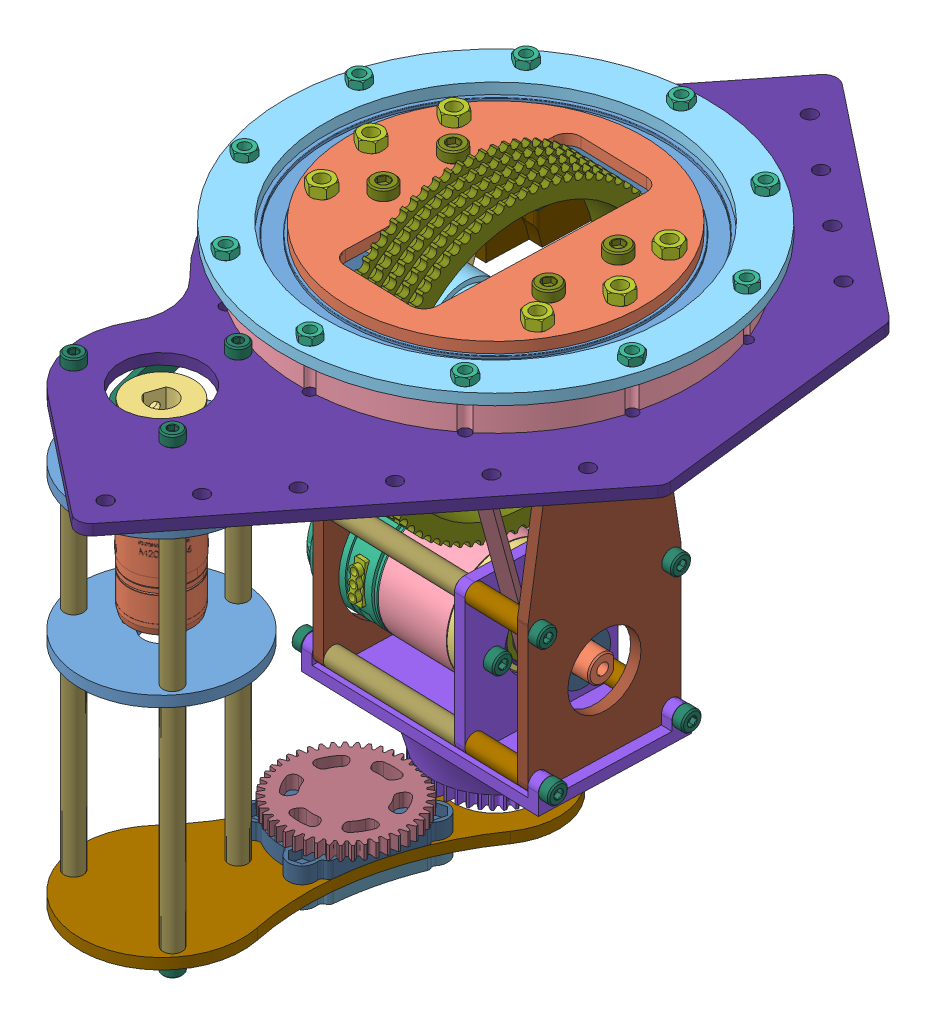
SolidWorks assembly 舵轮装配, configuration 默认. Lengths in mm.
Overall size (293.56 219.24 297.58).
150 component instances, 58 part files, 247 mates.
Components (placement in the parent):
- am-0198 4in Plaction Wheel-1: am-0198 4in Plaction Wheel [默认] at (-23.1352 -37.2288 84.5309) x (-0.999547 0 -0.03008) z (-0.012763 0.90552 0.424112)
  - am-0198 4in Plaction Wheel(2)^am-0198 4in Plaction Wheel-1: am-0198 4in Plaction Wheel(2)^am-0198 4in Plaction Wheel [默认] at origin (virtual)
- HRB 61821薄圈轴承-1: HRB 61821薄圈轴承 [默认] at (-8.689 -8.0564 92.8497) size (130 13 130)
- 舵轮底板-1: 舵轮底板 [默认] at (-8.689 4.9436 92.8497) x (-0.03008 0 0.999547) z (-0.999547 0 -0.03008) size (109 4 109)
- 舵轮侧面支撑-1: 舵轮侧面支撑 [默认] at (-38.1757 4.9436 91.9624) x (0.999547 0 0.03008) z (0.03008 0 -0.999547) size (14 45 35)
- 65齿 3m同步轮_舵轮定制板-1: 65齿 3m同步轮_舵轮定制板 [默认] at (11.9556 -30.0564 93.471) x (-0.028085 -0.358129 0.933249) z (0.999547 0 0.03008) size (62.3 62.3 8)
- 轮子轴承安装件-1: 轮子轴承安装件 [默认] at (-20.0339 -30.0564 92.5083) x (0.018247 -0.794989 -0.606349) z (0.023913 0.606624 -0.794629) size (28.1 11.65 28.1)
- 22 8 7轴承-1: 22 8 7轴承 [默认] at (-23.1825 -30.0564 92.4136) x (0.999547 0 0.03008) z (-0.028413 -0.328241 0.944167) size (7 25 25)
- 22 8 7轴承-2: 22 8 7轴承 [默认] at (12.9552 -30.0564 93.5011) x (-0.999547 0 -0.03008) z (0.029756 -0.146481 -0.988766) size (7 25 25)
- 舵轮用钢轴-1: 舵轮用钢轴 [默认] at (-43.1734 -30.0564 91.812) x (0.011091 0.929546 -0.368539) z (0.027961 -0.368706 -0.929125) size (8 70 8)
- 舵轮侧面支撑B-1: 舵轮侧面支撑B [默认] at (24.7958 4.9436 93.8574) x (-0.999547 0 -0.03008) z (-0.03008 0 0.999547) size (8 45 35)
- 舵轮轴承契合垫-1: 舵轮轴承契合垫 [默认] at (-8.689 -8.0564 92.8497) x (0.999547 0 0.03008) z (-0.03008 0 0.999547) size (18.69 13 65.65)
- 舵轮上底板-1: 舵轮上底板 [默认] at (-8.689 -12.0564 92.8497) x (-0.03008 0 0.999547) z (-0.999547 0 -0.03008) size (120 4 120)
- M3508电机安装板-1: M3508电机安装板 [默认] at (28.794 -7.5564 93.9777) x (0 1 0) z (0.03008 0 -0.999547) size (145.98 4 55)
- RoboMaster M3508直流无刷减速电-1: RoboMaster M3508直流无刷减速电 [默认] at (-82.126 -108.2793 108.2339) x (-0.011386 -0.925598 0.378336) z (0.999547 0 0.03008) size (77.46 77.46 98.4)
  - RoboMaster M3508直流无刷减速电 (1).STEP-1: RoboMaster M3508直流无刷减速电 (1).STEP [默认] at origin size (77.46 77.46 98.4)
    - 4_ASM_1.STEP-1: 4_ASM_1.STEP [默认] at (-1.7887 18.2683 39.841) x (-0.923508 0.383579 0) z (0.383579 0.923508 0) size (13.16 4.26 21.29)
      - __-__10_1__1.STEP-1: __-__10_1__1.STEP [默认] at origin size (2.4 2.3 2.24)
      - __-__10_3__1.STEP-1: __-__10_3__1.STEP [默认] at origin size (2.4 2.3 2.24)
      - __-__10_2__1.STEP-1: __-__10_2__1.STEP [默认] at origin size (2.4 2.3 2.24)
      - __-__20_1.STEP-1: __-__20_1.STEP [默认] at origin size (5.92 4.26 12.18)
    - 2_ASM.STEP-1: 2_ASM.STEP [默认] at (-1.7887 18.2683 50.441) x (-0.378508 0.925598 0) z (0.925598 0.378508 0) size (59.4 67.29 59.4)
      - 26_ASM.STEP-1: 26_ASM.STEP [默认] at (0 34.5 0) x (-0.381788 0 0.92425) z (-0.92425 0 -0.381788) size (22 6 22)
        - 28_1.STEP-1: 28_1.STEP [默认] at (0 2.5 0) size (20 0.2 20)
        - 27_1.STEP-1: 27_1.STEP [默认] at origin size (22 6 22)
        - 28_1.STEP-2: 28_1.STEP [默认] at (0 -2.7 0) size (20 0.2 20)
      - 26_ASM-1.STEP-1: 26_ASM-1.STEP [默认] at (0 27 0) x (-0.381788 0 0.92425) z (-0.92425 0 -0.381788) size (22 6 22)
        - 28_1.STEP-1: 28_1.STEP [默认] at (0 2.5 0) size (20 0.2 20)
        - 27_1.STEP-1: 27_1.STEP [默认] at origin size (22 6 22)
        - 28_1.STEP-2: 28_1.STEP [默认] at (0 -2.7 0) size (20 0.2 20)
      - 25_1.STEP-1: 25_1.STEP [默认] at (0 38.5 0) x (0 0 1) z (-1 0 0) size (16.7 1 13.43)
      - 18_1.STEP-1: 18_1.STEP [默认] at (-12.3744 22 -12.3744) x (0.381788 0 -0.92425) z (0.92425 0 0.381788) size (5.5 37.99 5.5)
      - 17_1.STEP-1: 17_1.STEP [默认] at (0 19.3 0) x (-1 0 0) z (0 0 -1) size (26 44 26)
      - 16_1.STEP-1: 16_1.STEP [默认] at (0 31 0) x (-0.707107 0 0.707107) z (0 1 0) size (42 42 14)
      - 18_1.STEP-2: 18_1.STEP [默认] at (12.3744 22 -12.3744) x (0.92425 0 0.381788) z (-0.381788 0 0.92425) size (5.5 37.99 5.5)
      - 23_1.STEP-1: 23_1.STEP [默认] at origin size (42.11 26 42)
      - 18_1.STEP-3: 18_1.STEP [默认] at (12.3744 22 12.3744) x (-0.381788 0 0.92425) z (-0.92425 0 -0.381788) size (5.5 37.99 5.5)
      - 18_1.STEP-4: 18_1.STEP [默认] at (-12.3744 22 12.3744) x (-0.92425 0 -0.381788) z (0.381788 0 -0.92425) size (5.5 37.99 5.5)
      - 24_1.STEP-1: 24_1.STEP [默认] at (0 37.71 0) x (0 1 0) z (0.381788 0 -0.92425) size (0.42 16 16)
    - 1_1_1.STEP-1: 1_1_1.STEP [默认] at (-1.7887 18.2683 48.441) x (0.923508 -0.383579 0) z (0 0 1) size (42 42 43.4)
    - 3_1.STEP-1: 3_1.STEP [默认] at (4.5067 -1.7659 43.091) x (0.299781 -0.954008 0) z (0.954008 0.299781 0) size (5.77 4 14.5)
- M3508电机安装延长-1: M3508电机安装延长 [默认] at (8.8031 -113.5384 93.3761) x (0 1 0) z (-0.03008 0 0.999547) size (55 4 55)
- 螺纹M4_长度20铝柱-1: 螺纹M4_长度20铝柱 [默认] at (9.525 -137.5384 69.387) x (-0.023176 -0.637485 0.770114) z (-0.019176 0.770463 0.637196) size (7 20 7)
- 螺纹M4_长度20铝柱-2: 螺纹M4_长度20铝柱 [默认] at (8.0811 -137.5384 117.3653) x (-0.023176 -0.637485 0.770114) z (-0.019176 0.770463 0.637196) size (7 20 7)
- 螺纹M4_长度20铝柱-3: 螺纹M4_长度20铝柱 [默认] at (9.525 -89.5384 69.387) x (-0.023176 -0.637485 0.770114) z (-0.019176 0.770463 0.637196) size (7 20 7)
- 螺纹M4_长度20铝柱-4: 螺纹M4_长度20铝柱 [默认] at (8.0811 -89.5384 117.3653) x (-0.023176 -0.637485 0.770114) z (-0.019176 0.770463 0.637196) size (7 20 7)
- 舵轮20齿M3508驱动同步轮-1: 舵轮20齿M3508驱动同步轮 [默认] at (19.5122 -113.5384 93.6984) x (-0.03008 0 0.999547) z (-0.999547 0 -0.03008) size (19.34 19.34 13.32)
- M3508电机安装板B-1: M3508电机安装板B [默认] at (-49.1707 -7.5564 91.6315) x (0 1 0) z (0.03008 0 -0.999547) size (145.98 4 55)
- 螺纹M4_长度50铝柱-1: 螺纹M4_长度50铝柱 [默认] at (-45.8944 -89.5384 115.741) x (-0.017103 -0.822624 0.568328) z (-0.024745 0.568585 0.822252) size (7 50 7)
- 螺纹M4_长度50铝柱-2: 螺纹M4_长度50铝柱 [默认] at (-45.8944 -137.5384 115.741) x (-0.017103 -0.822624 0.568328) z (-0.024745 0.568585 0.822252) size (7 50 7)
- 螺纹M4_长度50铝柱-3: 螺纹M4_长度50铝柱 [默认] at (-44.4506 -137.5384 67.7627) x (-0.017103 -0.822624 0.568328) z (-0.024745 0.568585 0.822252) size (7 50 7)
- 螺纹M4_长度50铝柱-4: 螺纹M4_长度50铝柱 [默认] at (-44.4506 -89.5384 67.7627) x (-0.017103 -0.822624 0.568328) z (-0.024745 0.568585 0.822252) size (7 50 7)
- 舵轮用100齿3m同步带-1: 舵轮用100齿3m同步带 [默认] at (12.5157 -113.5364 93.4759) x (-0.000004 1 0.000143) z (0.03008 0.000143 -0.999547) size (119.08 7 42.19)
- 舵轮轴承契合垫B-1: 舵轮轴承契合垫B [默认] at (-8.689 -8.0564 92.8497) x (-0.999547 0 -0.03008) z (0.03008 0 -0.999547) size (18.69 13 65.65)
- M4螺丝头-3: M4螺丝头 [默认] at (33.5141 -89.5384 70.1089) x (-0.00984 -0.944977 0.326989) z (-0.028425 0.327137 0.944549) size (7.2 4.15 7.2)
- M4螺丝头-4: M4螺丝头 [默认] at (32.0703 -89.5384 118.0872) x (-0.01003 -0.94277 0.333292) z (-0.028359 0.333443 0.942344) size (7.2 4.15 7.2)
- M4螺丝头-6: M4螺丝头 [默认] at (-49.8926 -89.5384 115.6206) x (-0.018672 0.784011 0.620466) z (-0.023583 -0.620747 0.783656) size (7.2 4.15 7.2)
- M4螺丝头-7: M4螺丝头 [默认] at (-48.4488 -89.5384 67.6424) x (-0.018672 0.784011 0.620466) z (-0.023583 -0.620747 0.783656) size (7.2 4.15 7.2)
- M4螺丝头-11: M4螺丝头 [默认] at (8.2767 -113.5384 110.8682) x (0.027176 0.428695 -0.90304) z (0.012895 -0.903449 -0.428501) size (7.2 4.15 7.2)
- M4螺丝头-12: M4螺丝头 [默认] at (8.8031 -131.0384 93.3761) x (0.027176 0.428695 -0.90304) z (0.012895 -0.903449 -0.428501) size (7.2 4.15 7.2)
- M4螺丝头-13: M4螺丝头 [默认] at (9.3295 -113.5384 75.8841) x (0.027176 0.428695 -0.90304) z (0.012895 -0.903449 -0.428501) size (7.2 4.15 7.2)
- M4螺丝头-14: M4螺丝头 [默认] at (8.8031 -96.0384 93.3761) x (0.027176 0.428695 -0.90304) z (0.012895 -0.903449 -0.428501) size (7.2 4.15 7.2)
- M5螺丝头-1: M5螺丝头 [默认] at (-49.0203 -0.0564 86.6338) x (-0.018761 0.781658 0.623426) z (-0.023512 -0.623708 0.781304) size (8.7 5.42 8.7)
- M5螺丝头-2: M5螺丝头 [默认] at (-49.3211 -0.0564 96.6292) x (-0.018761 0.781658 0.623426) z (-0.023512 -0.623708 0.781304) size (8.7 5.42 8.7)
- M5螺丝头-3: M5螺丝头 [默认] at (-49.4715 -15.0564 101.627) x (-0.018672 0.784011 0.620466) z (-0.023583 -0.620747 0.783656) size (8.7 5.42 8.7)
- M5螺丝头-4: M5螺丝头 [默认] at (-48.8699 -15.0564 81.636) x (-0.018672 0.784011 0.620466) z (-0.023583 -0.620747 0.783656) size (8.7 5.42 8.7)
- 舵轮直角安装架-1: 舵轮直角安装架 [默认] at (-8.689 -12.0564 92.8497) x (-0.620388 0 0.784295) z (-0.784295 0 -0.620388) size (222.67 4 198.17)
- 舵轮转向同步轮 75齿-3: 舵轮转向同步轮 75齿 [默认] at (-8.6606 -24.5564 92.6837) x (-0.03008 0 0.999547) z (0 1 0) size (120.22 120.22 12.5)
- 舵轮转向电机安装件-1: 舵轮转向电机安装件 [默认] at (-34.8056 -36.0564 190.3422) x (-0.620388 0 0.784295) z (-0.784295 0 -0.620388) size (60 4 60)
- RoboMaster M2006 P36直流无刷减速电机.step-2: RoboMaster M2006 P36直流无刷减速电机.step [默认] at (-18.0705 -65.9516 202.121) x (0.1159 0 0.993261) z (0 -1 0) size (36.5 37.99 64.81)
- 螺纹M4_长度20铝柱-5: 螺纹M4_长度20铝柱 [默认] at (-58.0411 -32.0564 199.5679) x (0.031165 0 -0.999514) z (0.999514 0 0.031165) size (7 20 7)
- 螺纹M4_长度20铝柱-6: 螺纹M4_长度20铝柱 [默认] at (-15.1983 -32.0564 205.8519) size (7 20 7)
- 螺纹M4_长度20铝柱-7: 螺纹M4_长度20铝柱 [默认] at (-31.1775 -32.0564 165.6069) size (7 20 7)
- 舵轮转向驱动同步轮15齿-1: 舵轮转向驱动同步轮15齿 [默认] at (-34.8056 -23.0564 190.3422) x (0.319867 0 -0.947462) z (0 1 0) size (23.73 23.73 12)
- M5螺丝头-7: M5螺丝头 [默认] at (-50.521 -19.5564 115.3516) x (-0.831036 0 -0.556218) z (-0.556218 0 0.831036) size (8.7 5.42 8.7)
- M5螺丝头-8: M5螺丝头 [默认] at (-56.1675 -19.5564 91.4209) x (-0.81436 0 -0.58036) z (-0.58036 0 0.81436) size (8.7 5.42 8.7)
- M5螺丝头-9: M5螺丝头 [默认] at (-49.0922 -19.5564 67.8731) x (-0.816979 0 -0.576667) z (-0.576667 0 0.816979) size (8.7 5.42 8.7)
- M5螺丝头-10: M5螺丝头 [默认] at (31.7142 -19.5564 117.8264) x (-0.799505 0 -0.600659) z (-0.600659 0 0.799505) size (8.7 5.42 8.7)
- M5螺丝头-11: M5螺丝头 [默认] at (38.7895 -19.5564 94.2785) x (-0.837169 0 -0.546944) z (-0.546944 0 0.837169) size (8.7 5.42 8.7)
- M5螺丝头-12: M5螺丝头 [默认] at (32.4914 -15.0564 104.0935) x (-0.010967 -0.931169 0.364423) z (-0.02801 0.364588 0.930748) size (8.7 5.42 8.7)
- M5螺丝头-13: M5螺丝头 [默认] at (33.143 -19.5564 70.3479) x (-0.841397 0 -0.540417) z (-0.540417 0 0.841397) size (8.7 5.42 8.7)
- M5螺丝头-14: M5螺丝头 [默认] at (33.093 -15.0564 84.1026) x (-0.014355 -0.878771 0.477027) z (-0.026433 0.477243 0.878374) size (8.7 5.42 8.7)
- 舵轮大轴承定位环-1: 舵轮大轴承定位环 [默认] at (-8.689 -8.0564 92.8497) x (0.046331 0 0.998926) z (-0.998926 0 0.046331) size (144.14 13 144.2)
- 轴承压住-1: 轴承压住 [默认] at (-8.689 4.9436 92.8497) x (-0.549671 0 0.835381) z (-0.835381 0 -0.549671) size (156 4 156)
- M4螺丝头-15: M4螺丝头 [默认] at (-53.7253 -12.0564 36.5458) x (-0.837169 0 -0.546944) z (-0.546944 0 0.837169) size (7.2 4.15 7.2)
- M4螺丝头-16: M4螺丝头 [默认] at (-12.0295 -12.0564 20.8272) x (-0.837169 0 -0.546944) z (-0.546944 0 0.837169) size (7.2 4.15 7.2)
- M4螺丝头-17: M4螺丝头 [默认] at (30.9423 -12.0564 32.6188) x (-0.837169 0 -0.546944) z (-0.546944 0 0.837169) size (7.2 4.15 7.2)
- M4螺丝头-18: M4螺丝头 [默认] at (58.7762 -12.0564 67.4165) x (-0.837169 0 -0.546944) z (-0.546944 0 0.837169) size (7.2 4.15 7.2)
- M4螺丝头-19: M4螺丝头 [默认] at (60.8408 -12.0564 111.9289) x (-0.837169 0 -0.546944) z (-0.546944 0 0.837169) size (7.2 4.15 7.2)
- M4螺丝头-20: M4螺丝头 [默认] at (36.3473 -12.0564 149.1537) x (-0.837169 0 -0.546944) z (-0.546944 0 0.837169) size (7.2 4.15 7.2)
- M4螺丝头-21: M4螺丝头 [默认] at (-5.3485 -12.0564 164.8723) x (-0.837169 0 -0.546944) z (-0.546944 0 0.837169) size (7.2 4.15 7.2)
- M4螺丝头-22: M4螺丝头 [默认] at (-48.3203 -12.0564 153.0807) x (-0.837169 0 -0.546944) z (-0.546944 0 0.837169) size (7.2 4.15 7.2)
- M4螺丝头-23: M4螺丝头 [默认] at (-76.1543 -12.0564 118.2829) x (-0.837169 0 -0.546944) z (-0.546944 0 0.837169) size (7.2 4.15 7.2)
- M4螺丝头-24: M4螺丝头 [默认] at (-78.2188 -12.0564 73.7705) x (-0.837169 0 -0.546944) z (-0.546944 0 0.837169) size (7.2 4.15 7.2)
- M4螺母-1: M4螺母 [默认] at (60.8408 8.9436 111.9289) x (0.881272 0 0.472609) z (-0.472609 0 0.881272) size (6.78 3.05 7.83)
- M4螺母-3: M4螺母 [默认] at (-5.3485 8.9436 164.8723) x (0.993898 0 0.110304) z (-0.110304 0 0.993898) size (6.78 3.05 7.83)
- M4螺母-4: M4螺母 [默认] at (-48.3203 8.9436 153.0807) x (0.999943 0 -0.01068) z (0.01068 0 0.999943) size (6.78 3.05 7.83)
- M4螺母-5: M4螺母 [默认] at (-76.1543 8.9436 118.2829) x (0.999991 0 -0.004285) z (0.004285 0 0.999991) size (6.78 3.05 7.83)
- M4螺母-6: M4螺母 [默认] at (-78.2188 8.9436 73.7705) size (6.78 3.05 7.83)
- M4螺母-7: M4螺母 [默认] at (-53.7253 8.9436 36.5458) size (6.78 3.05 7.83)
- M4螺母-8: M4螺母 [默认] at (-12.0295 8.9436 20.8272) x (0.973597 0 -0.228273) z (0.228273 0 0.973597) size (6.78 3.05 7.83)
- M4螺母-9: M4螺母 [默认] at (30.9423 8.9436 32.6188) size (6.78 3.05 7.83)
- M4螺母-10: M4螺母 [默认] at (58.7762 8.9436 67.4165) x (0.989058 0 0.147529) z (-0.147529 0 0.989058) size (6.78 3.05 7.83)
- M4螺母-11: M4螺母 [默认] at (36.3473 8.9436 149.1537) x (0.999002 0 -0.044676) z (0.044676 0 0.999002) size (6.78 3.05 7.83)
- M5螺丝头-15: M5螺丝头 [默认] at (24.4198 8.9436 106.3518) size (8.7 5.42 8.7)
- M5螺丝头-16: M5螺丝头 [默认] at (25.1718 8.9436 81.3631) size (8.7 5.42 8.7)
- M5螺丝头-17: M5螺丝头 [默认] at (-37.7997 8.9436 79.468) size (8.7 5.42 8.7)
- M5螺丝头-18: M5螺丝头 [默认] at (-38.5517 8.9436 104.4567) size (8.7 5.42 8.7)
- M4螺丝头-25: M4螺丝头 [默认] at (-15.1983 -8.0564 205.8519) x (0.999987 0 0.005127) z (-0.005127 0 0.999987) size (7.2 4.15 7.2)
- M4螺丝头-26: M4螺丝头 [默认] at (-58.0411 -8.0564 199.5679) x (1 0 0.000539) z (-0.000539 0 1) size (7.2 4.15 7.2)
- M4螺丝头-27: M4螺丝头 [默认] at (-31.1775 -8.0564 165.6069) x (0.999978 0 -0.006592) z (0.006592 0 0.999978) size (7.2 4.15 7.2)
- M5螺母-1: M5螺母 [默认] at (-49.0922 8.9436 67.8731) size (8 4 9.24)
- M5螺母-2: M5螺母 [默认] at (-56.1675 8.9436 91.4209) size (8 4 9.24)
- M5螺母-3: M5螺母 [默认] at (-50.521 8.9436 115.3516) size (8 4 9.24)
- M5螺母-4: M5螺母 [默认] at (31.7142 8.9436 117.8264) size (8 4 9.24)
- M5螺母-5: M5螺母 [默认] at (38.7895 8.9436 94.2785) size (8 4 9.24)
- M5螺母-6: M5螺母 [默认] at (33.143 8.9436 70.3479) x (0.941499 0 -0.337015) z (0.337015 0 0.941499) size (8 4 9.24)
- 螺纹M4_长度50铝柱-5: 螺纹M4_长度50铝柱 [默认] at (-58.0411 -86.0564 199.5679) x (0.999871 0 0.016069) z (-0.016069 0 0.999871) size (7 50 7)
- 螺纹M4_长度50铝柱-6: 螺纹M4_长度50铝柱 [默认] at (-15.1983 -86.0564 205.8519) x (0.99968 0 0.025305) z (-0.025305 0 0.99968) size (7 50 7)
- 螺纹M4_长度50铝柱-7: 螺纹M4_长度50铝柱 [默认] at (-31.1775 -86.0564 165.6069) x (0.999817 0 0.019127) z (-0.019127 0 0.999817) size (7 50 7)
- 舵轮转向电机安装件-2: 舵轮转向电机安装件 [默认] at (-34.8056 -90.0564 190.3422) x (0.989413 0 0.145124) z (-0.145124 0 0.989413) size (60 4 60)
- 舵轮线引导和角度定位3D打印件-1: 舵轮线引导和角度定位3D打印件 [默认] at (-8.3392 -141.0384 92.8603) x (-0.03008 0 0.999547) z (0.999547 0 0.03008) size (73.09 24 90.3)
- C620无刷电机调速器.STEP-1: C620无刷电机调速器.STEP [默认] at (-30.0294 -150.4384 92.2075) x (-0.999547 0 -0.03008) z (0.03008 0 -0.999547)
  - 9.STEP-1: 9.STEP [默认] at (63.0501 2 0) x (0 0 1) z (1 0 0) (suppressed, hidden)
  - 6.STEP-1: 6.STEP [默认] at (-2.2 39.826 -7.4409) x (0 -0.431667 0.902033) z (-1 0 0) (suppressed, hidden)
  - 7.STEP-1: 7.STEP [默认] at (-1.7 0.6 0) (suppressed, hidden)
  - 8.STEP-1: 8.STEP [默认] at (-1.7 -0.6 0) x (0 -1 0) z (0 0 1) (suppressed, hidden)
  - 2.STEP-1: 2.STEP [默认] at (15.6004 -0.6014 9.8) x (0 0 -1) z (0 1 0) (suppressed, hidden)
  - 5.STEP-1: 5.STEP [默认] at (16.6 -3.6 -10.7) x (-0.36263 0 0.931933) z (-0.931933 0 -0.36263) (suppressed, hidden)
  - 5.STEP-2: 5.STEP [默认] at (16.6 -3.6 10.7) (suppressed, hidden)
  - 5.STEP-3: 5.STEP [默认] at (-14.3 -3.6 10.7) (suppressed, hidden)
  - 5.STEP-4: 5.STEP [默认] at (-14.3 -3.6 -10.7) (suppressed, hidden)
  - 10.STEP-1: 10.STEP [默认] at (-177.4931 0.4104 -3.9137) x (1 0 0) z (0 -1 0) (suppressed, hidden)
- 理线和舵轮角度定位支撑-1: 理线和舵轮角度定位支撑 [默认] at (-34.8056 -174.0564 190.3422) x (0.965951 0 0.258726) z (-0.258726 0 0.965951) size (60 4 154.24)
- 舵轮角度定位第二齿轮轴承锁定-1: 舵轮角度定位第二齿轮轴承锁定 [默认] at (-20.3843 -164.0564 136.5001) x (-0.258726 0 0.965951) z (-0.965951 0 -0.258726) size (93.42 10.62 47)
- 6704zz轴承-1: 6704zz轴承 [默认] at (-20.3843 -170.0564 136.5001) x (0.99836 0 0.057256) z (-0.057256 0 0.99836) size (27 4 27)
- 螺纹M4_长度80铝柱-1: 螺纹M4_长度80铝柱 [默认] at (-15.1983 -170.0564 205.8519) size (7 80 7)
- 螺纹M4_长度80铝柱-2: 螺纹M4_长度80铝柱 [默认] at (-31.1775 -170.0564 165.6069) x (0.999699 0 0.024549) z (-0.024549 0 0.999699) size (7 80 7)
- 螺纹M4_长度80铝柱-3: 螺纹M4_长度80铝柱 [默认] at (-58.0411 -170.0564 199.5679) size (7 80 7)
- 舵轮角度定位第二齿轮-1: 舵轮角度定位第二齿轮 [默认] at (-20.3843 -163.5564 136.5001) x (0.49303 0 0.870012) z (0 1 0) size (50.24 50.45 15.5)
- M4螺丝头-28: M4螺丝头 [默认] at (-31.1775 -174.0564 165.6069) x (-0.821163 0 -0.570693) z (-0.570693 0 0.821163) size (7.2 4.15 7.2)
- M4螺丝头-29: M4螺丝头 [默认] at (-58.0411 -174.0564 199.5679) x (-0.837169 0 -0.546944) z (-0.546944 0 0.837169) size (7.2 4.15 7.2)
- M4螺丝头-30: M4螺丝头 [默认] at (-15.1983 -174.0564 205.8519) x (-0.817286 0 -0.576232) z (-0.576232 0 0.817286) size (7.2 4.15 7.2)
- M4螺丝头-31: M4螺丝头 [默认] at (-52.7468 -137.5384 67.513) x (-0.021149 -0.711114 0.702759) z (0.02139 -0.703077 -0.710792) size (7.2 4.15 7.2)
- M4螺丝头-32: M4螺丝头 [默认] at (36.0685 -137.5384 118.2075) x (0.025373 -0.537113 -0.843128) z (-0.016156 -0.84351 0.53687) size (7.2 4.15 7.2)
- M4螺丝头-33: M4螺丝头 [默认] at (37.5123 -137.5384 70.2292) x (-0.029877 0.115959 0.992805) z (0.003488 0.993254 -0.115907) size (7.2 4.15 7.2)
- M4螺丝头-34: M4螺丝头 [默认] at (-54.1907 -137.5384 115.4913) x (-0.021149 -0.711114 0.702759) z (0.02139 -0.703077 -0.710792) size (7.2 4.15 7.2)
- 舵轮角度定位AS5600支撑-1: 舵轮角度定位AS5600支撑 [默认] at (-20.3843 -174.0564 136.5001) x (-0.258726 0 0.965951) z (-0.965951 0 -0.258726) size (49.84 4 35.05)
- 舵轮转向同步带90齿5m-2: 舵轮转向同步带90齿5m [默认] at (-34.8056 -23.5564 190.3422) x (0.96529 0 0.261181) z (-0.261181 0 0.96529) size (124.22 10 176.93)
- 4in蓝丁晴胶圈-1: 4in蓝丁晴胶圈 [默认] at (2.5619 -30.0564 93.1883) x (0.012375 -0.911448 -0.411228) z (0.027416 0.411415 -0.911036) size (107.49 22.86 107.48)
Mates (geometry in assembly coordinates):
- 同心2: concentric aligned: cylinder of HRB 61821薄圈轴承-1 through (-8.689 4.9436 92.8497) axis (0 -1 0) radius 65; cylinder of 舵轮底板-1 through (-8.689 8.9436 92.8497) axis (0 -1 0) radius 54.5
- 平行1: parallel anti-aligned: plane of am-0198 4in Plaction Wheel-1/am-0198 4in Plaction Wheel(2)^am-0198 4in Plaction Wheel-1/4 Modular Half^am-0198 4in Plaction Wheel(2)_am-0198 4in Plaction Wheel-1 through (11.5504 -1.3061 106.9366) normal (0.999547 0 0.03008); plane of 舵轮底板-1 through (10.0815 4.9436 50.8954) normal (-0.999547 0 -0.03008)
- 重合3: coincident anti-aligned: plane of HRB 61821薄圈轴承-1 through (-8.689 4.9436 92.8497) normal (0 1 0); plane of 舵轮底板-1 through (-8.689 4.9436 92.8497) normal (0 -1 0)
- 同心3: concentric anti-aligned: cylinder of 舵轮底板-1 through (-38.5517 14.9436 104.4567) axis (0 -1 0) radius 2.6; cylinder of 舵轮侧面支撑-1 through (-38.5517 -5.0564 104.4567) axis (0 1 0) radius 2.1
- 重合4: coincident anti-aligned: plane of 舵轮底板-1 through (-8.689 4.9436 92.8497) normal (0 -1 0); plane of 舵轮侧面支撑-1 through (-38.1757 4.9436 91.9624) normal (0 1 0)
- 同心5: concentric anti-aligned: cylinder of 舵轮底板-1 through (-37.7997 14.9436 79.468) axis (0 -1 0) radius 2.6; cylinder of 舵轮侧面支撑-1 through (-37.7997 -5.0564 79.468) axis (0 1 0) radius 2.1
- 同心6: concentric aligned: cone of am-0198 4in Plaction Wheel-1/am-0198 4in Plaction Wheel(2)^am-0198 4in Plaction Wheel-1/4 Modular Half^am-0198 4in Plaction Wheel(2)_am-0198 4in Plaction Wheel-2 through (-29.6815 -30.0564 92.218) axis (0.999547 0 0.03008); cylinder of 舵轮侧面支撑-1 through (-77.158 -30.0564 90.7893) axis (0.999547 0 0.03008) radius 4.05
- 同心8: concentric aligned: cone of am-0198 4in Plaction Wheel-1/am-0198 4in Plaction Wheel(2)^am-0198 4in Plaction Wheel-1/4 Modular Half^am-0198 4in Plaction Wheel(2)_am-0198 4in Plaction Wheel-1 through (11.9556 -30.0564 93.471) axis (-0.999547 0 -0.03008); cylinder of 65齿 3m同步轮_舵轮定制板-1 through (19.952 -30.0564 93.7117) axis (-0.999547 0 -0.03008) radius 31.152
- 重合6: coincident anti-aligned: plane of am-0198 4in Plaction Wheel-1/am-0198 4in Plaction Wheel(2)^am-0198 4in Plaction Wheel-1/4 Modular Half^am-0198 4in Plaction Wheel(2)_am-0198 4in Plaction Wheel-1 through (11.5504 -1.3061 106.9366) normal (0.999547 0 0.03008); plane of 65齿 3m同步轮_舵轮定制板-1 through (12.766 -18.2001 66.5436) normal (-0.999547 0 -0.03008)
- 同心9: concentric aligned: cone of am-0198 4in Plaction Wheel-1/am-0198 4in Plaction Wheel(2)^am-0198 4in Plaction Wheel-1/4 Modular Half^am-0198 4in Plaction Wheel(2)_am-0198 4in Plaction Wheel-2 through (-29.6815 -30.0564 92.218) axis (0.999547 0 0.03008); cylinder of 轮子轴承安装件-1 through (-29.6795 -30.0564 92.2181) axis (0.999547 0 0.03008) radius 14.05
- 重合7: coincident anti-aligned: plane of am-0198 4in Plaction Wheel-1/am-0198 4in Plaction Wheel(2)^am-0198 4in Plaction Wheel-1/4 Modular Half^am-0198 4in Plaction Wheel(2)_am-0198 4in Plaction Wheel-2 through (-19.8515 -42.994 86.4488) normal (-0.999547 0 -0.03008); plane of 轮子轴承安装件-1 through (-20.0339 -30.0564 92.5083) normal (0.999547 0 0.03008)
- 同心10: concentric aligned: cylinder of 轮子轴承安装件-1 through (-29.6795 -30.0564 92.2181) axis (0.999547 0 0.03008) radius 11; cylinder of 22 8 7轴承-1 through (-23.1825 -30.0564 92.4136) axis (0.999547 0 0.03008) radius 11
- 重合8: coincident anti-aligned: plane of 轮子轴承安装件-1 through (-28.1802 -30.0564 92.2632) normal (-0.999547 0 -0.03008); plane of 22 8 7轴承-1 through (-28.1802 -30.0564 92.2632) normal (0.999547 0 0.03008)
- 距离1: distance = 1 mm anti-aligned: plane of 22 8 7轴承-1 through (-30.1793 -30.0564 92.203) normal (-0.999547 0 -0.03008); plane of 舵轮侧面支撑-1 through (-30.6524 -55.0564 74.6809) normal (0.999547 0 0.03008)
- 同心11: concentric anti-aligned: cylinder of 65齿 3m同步轮_舵轮定制板-1 through (17.9529 -30.0564 93.6515) axis (0.999547 0 0.03008) radius 13.15; cylinder of 22 8 7轴承-2 through (12.9552 -30.0564 93.5011) axis (-0.999547 0 -0.03008) radius 4
- 重合11: coincident anti-aligned: plane of 65齿 3m同步轮_舵轮定制板-1 through (17.9529 -30.0564 93.6515) normal (0.999547 0 0.03008); plane of 22 8 7轴承-2 through (17.9529 -30.0564 93.6515) normal (-0.999547 0 -0.03008)
- 同心12: concentric anti-aligned: cylinder of 舵轮侧面支撑-1 through (-77.158 -30.0564 90.7893) axis (0.999547 0 0.03008) radius 4.05; cylinder of 舵轮用钢轴-1 through (26.7949 -30.0564 93.9176) axis (-0.999547 0 -0.03008) radius 4
- 重合12: coincident aligned: plane of 舵轮侧面支撑-1 through (-43.1734 -30.0564 91.812) normal (0.999547 0 0.03008); circle of 舵轮用钢轴-1
- 同心13: concentric aligned: cylinder of 舵轮用钢轴-1 through (26.7949 -30.0564 93.9176) axis (-0.999547 0 -0.03008) radius 4; cylinder of 舵轮侧面支撑B-1 through (66.7768 -30.0564 95.1208) axis (-0.999547 0 -0.03008) radius 4.05
- 同心14: concentric anti-aligned: cylinder of 舵轮侧面支撑B-1 through (24.4198 -5.0564 106.3518) axis (0 1 0) radius 2.1; cylinder of 舵轮底板-1 through (24.4198 104.9436 106.3518) axis (0 -1 0) radius 2.6
- 同心15: concentric aligned: cylinder of 舵轮底板-1 through (-56.1675 14.9436 91.4209) axis (0 -1 0) radius 2.6; cylinder of 舵轮轴承契合垫-1 through (-56.1675 4.9436 91.4209) axis (0 -1 0) radius 2.6
- 同心16: concentric aligned: cylinder of 舵轮底板-1 through (-50.521 14.9436 115.3516) axis (0 -1 0) radius 2.6; cylinder of 舵轮轴承契合垫-1 through (-50.521 4.9436 115.3516) axis (0 -1 0) radius 2.6
- 重合14: coincident anti-aligned: plane of 舵轮轴承契合垫-1 through (-8.689 4.9436 92.8497) normal (0 1 0); plane of 舵轮底板-1 through (-8.689 4.9436 92.8497) normal (0 -1 0)
- 同心19: concentric aligned: cylinder of HRB 61821薄圈轴承-1 through (-8.689 4.9436 92.8497) axis (0 -1 0) radius 65; cylinder of 舵轮上底板-1 through (-8.689 161.6493 92.8497) axis (0 -1 0) radius 60
- 重合16: coincident anti-aligned: plane of HRB 61821薄圈轴承-1 through (-8.689 -8.0564 92.8497) normal (0 -1 0); plane of 舵轮上底板-1 through (-8.689 -8.0564 92.8497) normal (0 1 0)
- 同心21: concentric anti-aligned: cylinder of 舵轮侧面支撑-1 through (-131.284 -0.0564 94.1627) axis (0.999547 0 0.03008) radius 2.1; cylinder of M3508电机安装板-1 through (32.6418 -0.0564 99.0958) axis (-0.999547 0 -0.03008) radius 2.6
- 同心22: concentric anti-aligned: cylinder of 舵轮侧面支撑-1 through (-131.4344 -15.0564 99.1604) axis (0.999547 0 0.03008) radius 2.1; cylinder of M3508电机安装板-1 through (32.4914 -15.0564 104.0935) axis (-0.999547 0 -0.03008) radius 2.6
- 重合17: coincident anti-aligned: plane of 舵轮侧面支撑B-1 through (28.794 -30.0564 93.9777) normal (0.999547 0 0.03008); plane of M3508电机安装板-1 through (28.794 -7.5564 93.9777) normal (-0.999547 0 -0.03008)
- 同心23: concentric anti-aligned: cylinder of M3508电机安装板-1 through (22.7967 -113.5384 93.7973) axis (0.999547 0 0.03008) radius 13.15; circle of RoboMaster M3508直流无刷减速电-1/2_ASM-1/16_1-1
- 同心24: concentric anti-aligned: cylinder of M3508电机安装板-1 through (22.0748 -89.5384 117.7864) axis (0.999547 0 0.03008) radius 2.1; cylinder of M3508电机安装延长-1 through (8.0811 -89.5384 117.3653) axis (-0.999547 0 -0.03008) radius 2.1
- 同心25: concentric anti-aligned: cylinder of M3508电机安装板-1 through (22.7967 -113.5384 93.7973) axis (0.999547 0 0.03008) radius 13.15; cylinder of M3508电机安装延长-1 through (8.8031 -113.5384 93.3761) axis (-0.999547 0 -0.03008) radius 13.15
- 重合18: coincident anti-aligned: plane of RoboMaster M3508直流无刷减速电-1/2_ASM-1/16_1-1 through (4.5284 -104.346 102.4441) normal (0.999547 0 0.03008); plane of M3508电机安装延长-1 through (4.8049 -113.5384 93.2558) normal (-0.999547 0 -0.03008)
- 同心27: concentric anti-aligned: cylinder of M3508电机安装板-1 through (23.5186 -137.5384 69.8081) axis (0.999547 0 0.03008) radius 2.1; cylinder of 螺纹M4_长度20铝柱-1 through (29.5159 -137.5384 69.9886) axis (-0.999547 0 -0.03008) radius 3.5
- 重合19: coincident anti-aligned: plane of M3508电机安装板-1 through (28.794 -7.5564 93.9777) normal (-0.999547 0 -0.03008); plane of 螺纹M4_长度20铝柱-1 through (29.5159 -137.5384 69.9886) normal (0.999547 0 0.03008)
- 重合20: coincident anti-aligned: plane of M3508电机安装延长-1 through (8.8031 -113.5384 93.3761) normal (0.999547 0 0.03008); plane of 螺纹M4_长度20铝柱-1 through (9.525 -137.5384 69.387) normal (-0.999547 0 -0.03008)
- 同心29: concentric anti-aligned: cylinder of M3508电机安装板-1 through (23.5186 -89.5384 69.8081) axis (0.999547 0 0.03008) radius 2.1; cylinder of 螺纹M4_长度20铝柱-3 through (29.5159 -89.5384 69.9886) axis (-0.999547 0 -0.03008) radius 3.5
- 同心30: concentric anti-aligned: cylinder of M3508电机安装板-1 through (22.0748 -89.5384 117.7864) axis (0.999547 0 0.03008) radius 2.1; cylinder of 螺纹M4_长度20铝柱-4 through (28.0721 -89.5384 117.9669) axis (-0.999547 0 -0.03008) radius 3.5
- 同心31: concentric anti-aligned: cylinder of M3508电机安装板-1 through (22.0748 -137.5384 117.7864) axis (0.999547 0 0.03008) radius 2.1; cylinder of 螺纹M4_长度20铝柱-2 through (28.0721 -137.5384 117.9669) axis (-0.999547 0 -0.03008) radius 3.5
- 重合21: coincident anti-aligned: plane of M3508电机安装板-1 through (28.794 -7.5564 93.9777) normal (-0.999547 0 -0.03008); plane of 螺纹M4_长度20铝柱-2 through (28.0721 -137.5384 117.9669) normal (0.999547 0 0.03008)
- 重合22: coincident anti-aligned: plane of M3508电机安装延长-1 through (8.8031 -113.5384 93.3761) normal (0.999547 0 0.03008); plane of 螺纹M4_长度20铝柱-4 through (8.0811 -89.5384 117.3653) normal (-0.999547 0 -0.03008)
- 重合23: coincident anti-aligned: plane of M3508电机安装板-1 through (28.794 -7.5564 93.9777) normal (-0.999547 0 -0.03008); plane of 螺纹M4_长度20铝柱-3 through (29.5159 -89.5384 69.9886) normal (0.999547 0 0.03008)
- 同心32: concentric anti-aligned: cylinder of RoboMaster M3508直流无刷减速电-1/2_ASM-1/17_1-1 through (32.0925 -113.5384 94.077) axis (0.999547 0 0.03008) radius 5; cylinder of 舵轮20齿M3508驱动同步轮-1 through (19.5122 -113.5384 93.6984) axis (-0.999547 0 -0.03008) radius 5.15
- 距离2: distance = 4.88 mm aligned: plane of 65齿 3m同步轮_舵轮定制板-1 through (19.952 -30.0564 93.7117) normal (0.999547 0 0.03008); plane of 舵轮20齿M3508驱动同步轮-1 through (24.8298 -113.5384 93.8584) normal (0.999547 0 0.03008)
- 重合27: coincident anti-aligned: plane of 舵轮侧面支撑-1 through (-44.6461 -55.0564 74.2597) normal (-0.999547 0 -0.03008); plane of M3508电机安装板B-1 through (-45.1725 -7.5564 91.7518) normal (0.999547 0 0.03008)
- 同心36: concentric anti-aligned: cylinder of 舵轮侧面支撑-1 through (-130.8328 -15.0564 79.1695) axis (0.999547 0 0.03008) radius 2.1; cylinder of M3508电机安装板B-1 through (-44.8717 -15.0564 81.7563) axis (-0.999547 0 -0.03008) radius 2.6
- 同心37: concentric anti-aligned: cylinder of 舵轮侧面支撑-1 through (-131.4344 -15.0564 99.1604) axis (0.999547 0 0.03008) radius 2.1; cylinder of M3508电机安装板B-1 through (-45.4733 -15.0564 101.7473) axis (-0.999547 0 -0.03008) radius 2.6
- 同心39: concentric anti-aligned: cylinder of M3508电机安装板B-1 through (-54.4461 -137.5384 67.4619) axis (0.999547 0 0.03008) radius 2.1; cylinder of 螺纹M4_长度50铝柱-3 through (5.5268 -137.5384 69.2667) axis (-0.999547 0 -0.03008) radius 3.5
- 同心40: concentric anti-aligned: cylinder of M3508电机安装板B-1 through (-55.8899 -137.5384 115.4402) axis (0.999547 0 0.03008) radius 2.1; cylinder of 螺纹M4_长度50铝柱-2 through (4.083 -137.5384 117.245) axis (-0.999547 0 -0.03008) radius 3.5
- 同心41: concentric anti-aligned: cylinder of M3508电机安装板B-1 through (-55.8899 -89.5384 115.4402) axis (0.999547 0 0.03008) radius 2.1; cylinder of 螺纹M4_长度50铝柱-1 through (4.083 -89.5384 117.245) axis (-0.999547 0 -0.03008) radius 3.5
- 同心42: concentric anti-aligned: cylinder of M3508电机安装板B-1 through (-54.4461 -89.5384 67.4619) axis (0.999547 0 0.03008) radius 2.1; cylinder of 螺纹M4_长度50铝柱-4 through (5.5268 -89.5384 69.2667) axis (-0.999547 0 -0.03008) radius 3.5
- 重合28: coincident anti-aligned: plane of M3508电机安装板B-1 through (-45.1725 -7.5564 91.7518) normal (0.999547 0 0.03008); plane of 螺纹M4_长度50铝柱-2 through (-45.8944 -137.5384 115.741) normal (-0.999547 0 -0.03008)
- 重合29: coincident anti-aligned: plane of M3508电机安装延长-1 through (4.8049 -113.5384 93.2558) normal (-0.999547 0 -0.03008); plane of 螺纹M4_长度50铝柱-3 through (5.5268 -137.5384 69.2667) normal (0.999547 0 0.03008)
- 重合30: coincident anti-aligned: plane of M3508电机安装板B-1 through (-45.1725 -7.5564 91.7518) normal (0.999547 0 0.03008); plane of 螺纹M4_长度50铝柱-1 through (-45.8944 -89.5384 115.741) normal (-0.999547 0 -0.03008)
- 重合31: coincident anti-aligned: plane of M3508电机安装板B-1 through (-45.1725 -7.5564 91.7518) normal (0.999547 0 0.03008); plane of 螺纹M4_长度50铝柱-4 through (-44.4506 -89.5384 67.7627) normal (-0.999547 0 -0.03008)
- 重合32: coincident anti-aligned: plane of 舵轮20齿M3508驱动同步轮-1 through (19.5122 -113.5384 93.6984) normal (-0.999547 0 -0.03008); plane of 舵轮用100齿3m同步带-1 through (19.5126 -113.5364 93.6865) normal (0.999547 0 0.03008)
- 同心53: concentric aligned: cylinder of 65齿 3m同步轮_舵轮定制板-1 through (19.952 -30.0564 93.7117) axis (-0.999547 0 -0.03008) radius 31.152; cylinder of 舵轮用100齿3m同步带-1 through (19.5122 -30.0564 93.6984) axis (-0.999547 0 -0.03008) radius 12.5
- 锁定1: lock: unknown of 舵轮20齿M3508驱动同步轮-1; unknown of 舵轮用100齿3m同步带-1
- 同心56: concentric aligned: cylinder of 舵轮底板-1 through (38.7895 14.9436 94.2785) axis (0 -1 0) radius 2.6; cylinder of 舵轮轴承契合垫B-1 through (38.7895 4.9436 94.2785) axis (0 -1 0) radius 2.6
- 同心57: concentric aligned: cylinder of 舵轮底板-1 through (33.143 14.9436 70.3479) axis (0 -1 0) radius 2.6; cylinder of 舵轮轴承契合垫B-1 through (33.143 4.9436 70.3479) axis (0 -1 0) radius 2.6
- 重合34: coincident anti-aligned: plane of 舵轮底板-1 through (-8.689 4.9436 92.8497) normal (0 -1 0); plane of 舵轮轴承契合垫B-1 through (-8.689 4.9436 92.8497) normal (0 1 0)
- 同心59: concentric anti-aligned: cylinder of M4螺丝头-3 through (37.5123 -89.5384 70.2292) axis (-0.999547 0 -0.03008) radius 3.6; cylinder of M3508电机安装板-1 through (23.5186 -89.5384 69.8081) axis (0.999547 0 0.03008) radius 2.1
- 同心60: concentric anti-aligned: cylinder of M3508电机安装板-1 through (22.0748 -89.5384 117.7864) axis (0.999547 0 0.03008) radius 2.1; cylinder of M4螺丝头-4 through (36.0685 -89.5384 118.2075) axis (-0.999547 0 -0.03008) radius 3.6
- 重合37: coincident anti-aligned: plane of M3508电机安装板-1 through (32.7922 -7.5564 94.0981) normal (0.999547 0 0.03008); plane of M4螺丝头-4 through (32.0703 -89.5384 118.0872) normal (-0.999547 0 -0.03008)
- 重合38: coincident anti-aligned: plane of M3508电机安装板-1 through (32.7922 -7.5564 94.0981) normal (0.999547 0 0.03008); plane of M4螺丝头-3 through (33.5141 -89.5384 70.1089) normal (-0.999547 0 -0.03008)
- 重合41: coincident anti-aligned: plane of M3508电机安装板B-1 through (-49.1707 -7.5564 91.6315) normal (-0.999547 0 -0.03008); plane of M4螺丝头-7 through (-48.4488 -89.5384 67.6424) normal (0.999547 0 0.03008)
- 同心64: concentric aligned: cylinder of M3508电机安装板B-1 through (-54.4461 -89.5384 67.4619) axis (0.999547 0 0.03008) radius 2.1; cylinder of M4螺丝头-7 through (-52.447 -89.5384 67.522) axis (0.999547 0 0.03008) radius 3.6
- 重合42: coincident anti-aligned: plane of M3508电机安装板B-1 through (-49.1707 -7.5564 91.6315) normal (-0.999547 0 -0.03008); plane of M4螺丝头-6 through (-49.8926 -89.5384 115.6206) normal (0.999547 0 0.03008)
- 同心65: concentric aligned: cylinder of M3508电机安装板B-1 through (-55.8899 -89.5384 115.4402) axis (0.999547 0 0.03008) radius 2.1; cylinder of M4螺丝头-6 through (-53.8908 -89.5384 115.5003) axis (0.999547 0 0.03008) radius 3.6
- 同心66: concentric aligned: cylinder of M3508电机安装延长-1 through (8.2767 -113.5384 110.8682) axis (-0.999547 0 -0.03008) radius 2.1; cylinder of M4螺丝头-11 through (12.2749 -113.5384 110.9885) axis (-0.999547 0 -0.03008) radius 3.6
- 同心67: concentric aligned: cylinder of M3508电机安装延长-1 through (8.8031 -131.0384 93.3761) axis (-0.999547 0 -0.03008) radius 2.1; cylinder of M4螺丝头-12 through (12.8013 -131.0384 93.4965) axis (-0.999547 0 -0.03008) radius 3.6
